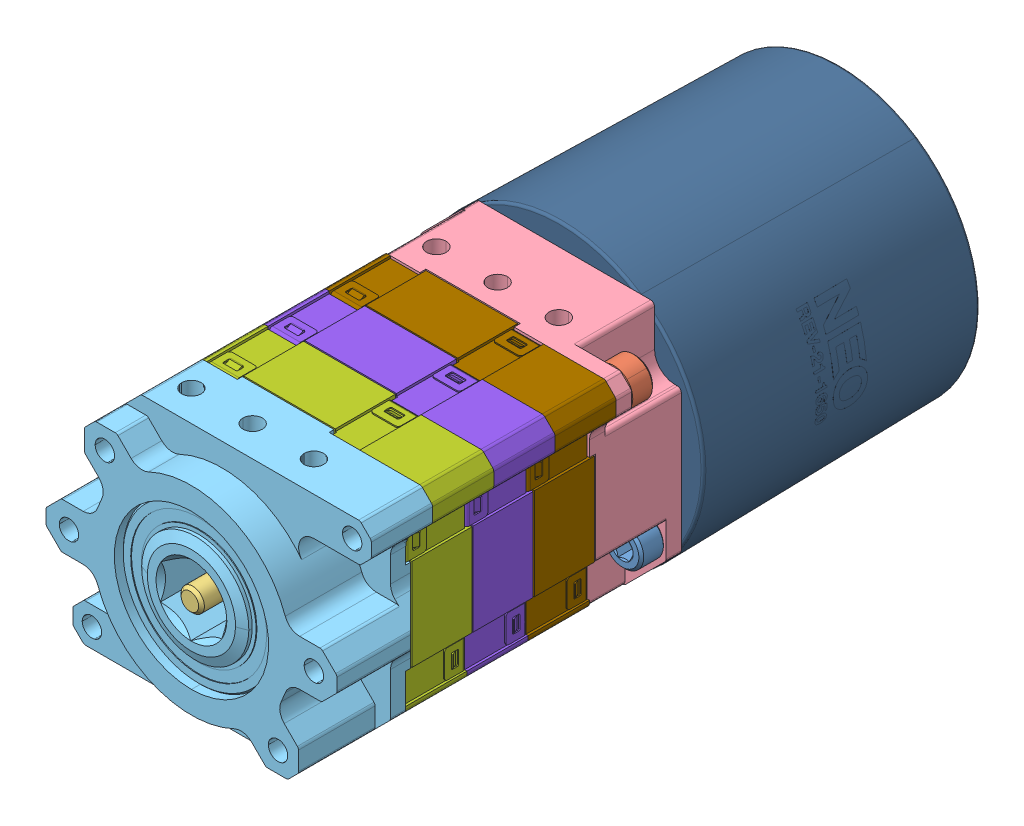
SolidWorks assembly MAXPlanetary 3-Stage, configuration Default. Lengths in mm.
Overall size (89.61 89.51 134.78).
15 component instances, 10 part files, 0 mates.
Components (placement in the parent):
- MAXPlanetary 3-Stage.STEP-1: MAXPlanetary 3-Stage.STEP [Default] at origin size (89.61 89.51 134.78)
  - REV-25-2109_3-Stage (No Shaft, For NEO).STEP-1: REV-25-2109_3-Stage (No Shaft, For NEO).STEP [Default] at origin size (65.21 54.09 86.04)
    - REV-25-2107_3-Stage.STEP-1: REV-25-2107_3-Stage.STEP [Default] at (0 0 6.35) x (-1 0 0) z (0 0 -1) size (65.21 54.09 86.04)
      - #10 Socket Head Cap Screws_0.500in Long.STEP-1: #10 Socket Head Cap Screws_0.500in Long.STEP [Default] at (21.1355 14.0872 12.7) x (0.923728 0.383049 0) z (0.383049 -0.923728 0) size (7.94 17.53 7.94)
      - #10 Socket Head Cap Screws_0.500in Long.STEP-2: #10 Socket Head Cap Screws_0.500in Long.STEP [Default] at (-21.1355 -14.0872 12.7) x (0.923728 0.383049 0) z (0.383049 -0.923728 0) size (7.94 17.53 7.94)
      - #10 Socket Head Cap Screws_2.000in Long.STEP-1: #10 Socket Head Cap Screws_2.000in Long.STEP [Default] at (-26.9919 21.4312 0) x (0.715577 0.698533 0) z (-0.698533 0.715577 0) size (7.94 55.63 7.94)
      - #10 Socket Head Cap Screws_2.000in Long.STEP-2: #10 Socket Head Cap Screws_2.000in Long.STEP [Default] at (26.9919 -21.4312 0) x (0.715577 0.698533 0) z (-0.698533 0.715577 0) size (7.94 55.63 7.94)
      - #10-32 Button Head Cap Screws_0.500in Long.STEP-1: #10-32 Button Head Cap Screws_0.500in Long.STEP [Default] at (0 0 -47.9425) x (0.655967 -0.754789 0) z (-0.754789 -0.655967 0) size (9.17 15.27 9.17)
    - REV-21-2106.STEP-1: REV-21-2106.STEP [Default] at origin size (61.91 50.8 19.05)
    - REV-21-2104.STEP-1: REV-21-2104.STEP [Default] at (0 0 57.15) x (0 0 1) z (-1 0 0) size (23.2 50.8 61.92)
    - REV-21-2108.STEP-1: REV-21-2108.STEP [Default] at (0 0 7.0985) x (-0.554615 -0.832107 0) z (0 0 -1) size (25.4 25.4 14.94)
  - REV-21-2101.STEP-1: REV-21-2101.STEP [Default] at (0 0 41.275) size (61.91 50.8 16.85)
  - REV-21-2102.STEP-1: REV-21-2102.STEP [Default] at (0 0 28.575) size (61.91 50.8 17.5)
  - REV-21-2103.STEP-1: REV-21-2103.STEP [Default] at (0 0 15.875) size (61.91 50.8 16.85)
  - REV-21-1650.STEP-1: REV-21-1650.STEP [Default] at (0 0 -9.525) x (0.554615 0.832107 0) z (0 0 1) size (64.41 64.76 93.26)
